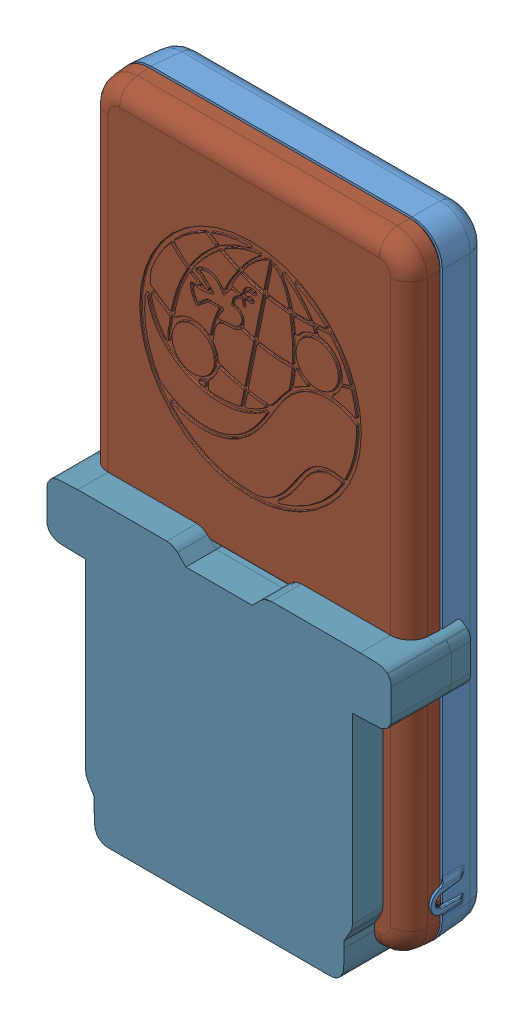
SolidWorks assembly pcb assm new, configuration Default. Lengths in mm.
Overall size (86.92 165.02 40.71).
43 component instances, 14 part files, 21 mates.
Components (placement in the parent):
- pcb top new-1: pcb top new [Default] at origin size (86.92 165 16.48)
- pcb w pot-1: pcb w pot [Default] at (-73.5 149.8449 0.1) x (0 -1 0) z (0 0 -1) size (61 49 35.64)
  - pcb w pot.step-1: pcb w pot.step [Default] at origin size (61 49 48.39)
    - DIP-8_W7.62mm.step-1: DIP-8_W7.62mm.step [Default] at (118.872 -61.849 1.65) x (0 -1 0) z (0 0 1) size (7.87 9.27 6.98)
      - SOLID.step-1: SOLID.step [Default] at origin size (7.87 9.27 6.98)
    - PTV09A-4030S-A503.step-1: PTV09A-4030S-A503.step [Default] at (115.189 -83.439 1.65) x (0 1 0) z (0 0 1) size (11.44 12.9 35.6)
      - COMPOUND.step-1: COMPOUND.step [Default] at origin size (11.44 12.9 35.6)
    - R_0805_2012Metric.step-1: R_0805_2012Metric.step [Default] at (112.411 -57.658 1.65) size (2 1.2 0.45)
      - SOLID-0.step-1: SOLID-0.step [Default] at origin size (2 1.2 0.45)
    - R_0805_2012Metric.step-2: R_0805_2012Metric.step [Default] at (121.682 -90.932 1.65) x (0 -1 0) z (0 0 1) size (2 1.2 0.45)
      - SOLID-0.step-1: SOLID-0.step [Default] at origin size (2 1.2 0.45)
    - R_0805_2012Metric.step-3: R_0805_2012Metric.step [Default] at (121.142 -85.979 1.65) x (-1 0 0) z (0 0 1) size (2 1.2 0.45)
      - SOLID-0.step-1: SOLID-0.step [Default] at origin size (2 1.2 0.45)
    - R_0805_2012Metric.step-4: R_0805_2012Metric.step [Default] at (117.364 -57.658 1.65) size (2 1.2 0.45)
      - SOLID-0.step-1: SOLID-0.step [Default] at origin size (2 1.2 0.45)
    - R_0805_2012Metric.step-5: R_0805_2012Metric.step [Default] at (127 -80.772 1.65) x (-1 0 0) z (0 0 1) size (2 1.2 0.45)
      - SOLID-0.step-1: SOLID-0.step [Default] at origin size (2 1.2 0.45)
    - R_Axial_DIN0207_L6.3mm_D2.5mm_P7.62mm_Horizontal.step-1: R_Axial_DIN0207_L6.3mm_D2.5mm_P7.62mm_Horizontal.step [Default] at (105.537 -92.583 1.65) size (8.22 2.5 5.5)
      - SOLID-1.step-1: SOLID-1.step [Default] at origin size (8.22 2.5 5.5)
    - R_0805_2012Metric.step-6: R_0805_2012Metric.step [Default] at (88.265 -82.534 1.65) x (0 -1 0) z (0 0 1) size (2 1.2 0.45)
      - SOLID-0.step-1: SOLID-0.step [Default] at origin size (2 1.2 0.45)
    - R_Axial_DIN0204_L3.6mm_D1.6mm_P2.54mm_Vertical.step-1: R_Axial_DIN0204_L3.6mm_D1.6mm_P2.54mm_Vertical.step [Default] at (137.668 -93.726 1.65) x (0 1 0) z (0 0 1) size (3.59 1.6 9.6)
      - SOLID-2.step-1: SOLID-2.step [Default] at origin size (3.59 1.6 9.6)
    - R_Axial_DIN0204_L3.6mm_D1.6mm_P2.54mm_Vertical.step-2: R_Axial_DIN0204_L3.6mm_D1.6mm_P2.54mm_Vertical.step [Default] at (132.334 -91.44 1.65) x (0 -1 0) z (0 0 1) size (3.59 1.6 9.6)
      - SOLID-2.step-1: SOLID-2.step [Default] at origin size (3.59 1.6 9.6)
    - LM317MABTG.step-1: LM317MABTG.step [Default] at (95.377 -83.058 1.65) x (0 1 0) z (0 0 1) size (9.97 4.82 36.27)
      - COMPOUND-3.step-1: COMPOUND-3.step [Default] at origin size (9.97 4.82 36.27)
    - C_0805_2012Metric.step-1: C_0805_2012Metric.step [Default] at (118.364 -95.25 1.65) x (0 -1 0) z (0 0 1) size (2 1.25 1.25)
      - SOLID-4.step-1: SOLID-4.step [Default] at origin size (2 1.25 1.25)
    - C_0805_2012Metric.step-2: C_0805_2012Metric.step [Default] at (109.855 -52.832 1.65) x (0 1 0) z (0 0 1) size (2 1.25 1.25)
      - SOLID-4.step-1: SOLID-4.step [Default] at origin size (2 1.25 1.25)
    - C_1206_3216Metric.step-1: C_1206_3216Metric.step [Default] at (121.285 -80.772 1.65) x (-1 0 0) z (0 0 1) size (3.2 1.6 1.6)
      - SOLID-5.step-1: SOLID-5.step [Default] at origin size (3.2 1.6 1.6)
    - C_0805_2012Metric.step-3: C_0805_2012Metric.step [Default] at (88.392 -76.3485 1.65) x (0 1 0) z (0 0 1) size (2 1.25 1.25)
      - SOLID-4.step-1: SOLID-4.step [Default] at origin size (2 1.25 1.25)
    - COMPOUND-6.step-1: COMPOUND-6.step [Default] at origin size (61 49 1.6)
- pcb bottom new-1: pcb bottom new [Default] at origin size (86.85 165 8.73)
- battery case-1: battery case [Default] at (0 -42.734 -10) size (59.56 61.47 15.11)
- Batteria ricaricabile stilo-1: Batteria ricaricabile stilo [Default] at (23.86 -20.0965 -1.9855) x (0 0 1) z (-1 0 0) size (13.97 13.97 50.04)
- Batteria ricaricabile stilo-2: Batteria ricaricabile stilo [Default] at (-23.86 -35.162 -1.9855) x (0 0 -1) z (1 0 0) size (13.97 13.97 50.04)
- Batteria ricaricabile stilo-3: Batteria ricaricabile stilo [Default] at (23.86 -50.2275 -1.872) x (0 0 1) z (-1 0 0) size (13.97 13.97 50.04)
- Batteria ricaricabile stilo-4: Batteria ricaricabile stilo [Default] at (-23.86 -65.3715 -1.9855) x (0 0 -1) z (1 0 0) size (13.97 13.97 50.04)
- pcb battery cover-1: pcb battery cover [Default] at origin size (91.07 78.3 21.02)
Mates (geometry in assembly coordinates):
- Coincident1: coincident anti-aligned: plane of pcb top new-1 through (0 0 -1.6) normal (0 0 1); plane of pcb w pot-1/pcb w pot.step-1/COMPOUND-6.step-1 through (0 36.3711 0) normal (0 0 1)
- Coincident2: coincident anti-aligned: plane of pcb top new-1 through (0 0 -1.5) normal (0 0 1); plane of pcb w pot-1/pcb w pot.step-1/COMPOUND-6.step-1 through (0 36.3449 -1.5) normal (0 0 -1)
- Width4: width aligned: plane of pcb bottom new-1 through (42.5 -82.5 0) normal (0.99863 0 0.052336); plane of pcb top new-1 through (-42.5 -82.5 0) normal (-0.99863 0 0.052336); plane of pcb bottom new-1 through (42.5 -82.5 0) normal (0.99863 0 -0.052336); plane of pcb top new-1 through (-42.5 -82.5 0) normal (-0.99863 0 -0.052336)
- Width5: width anti-aligned: plane of pcb bottom new-1 through (42.5 82.5 0) normal (0 0.99863 0.052336); plane of pcb top new-1 through (42.5 -82.5 0) normal (0 -0.99863 0.052336); plane of pcb bottom new-1 through (42.5 -82.5 0) normal (0 -0.99863 -0.052336); plane of pcb top new-1 through (42.5 82.5 0) normal (0 0.99863 -0.052336)
- Coincident3: coincident anti-aligned: plane of pcb top new-1 through (0 0 0) normal (0 0 1); plane of pcb bottom new-1 through (0 0 0) normal (0 0 -1)
- Width6: width aligned: plane of pcb w pot-1/pcb w pot.step-1/COMPOUND-6.step-1 through (-24.5 5.8449 0.1) normal (0 -1 0); plane of pcb top new-1 through (24.5 66.8449 0.1) normal (0 1 0); plane of pcb w pot-1/pcb w pot.step-1/COMPOUND-6.step-1 through (25.25 5.0949 -1.5) normal (0 0.99863 0.052336); plane of pcb top new-1 through (25.25 67.5949 -1.5) normal (0 -0.99863 0.052336)
- Width7: width aligned: plane of pcb w pot-1/pcb w pot.step-1/COMPOUND-6.step-1 through (24.5 5.8449 0.1) normal (1 0 0); plane of pcb top new-1 through (-24.5 66.8449 0.1) normal (-1 0 0); plane of pcb w pot-1/pcb w pot.step-1/COMPOUND-6.step-1 through (25.25 61.7904 -1.5) normal (-0.99863 0 0.052336); plane of pcb top new-1 through (-25.25 5.0949 -1.5) normal (0.99863 0 0.052336)
- Width8: width aligned: plane of battery case-1 through (-28.448 -12 5.113) normal (-1 0 0); plane of pcb top new-1 through (28.448 -12 5.113) normal (1 0 0); plane of battery case-1 through (42.5 -82.5 0) normal (0.99863 0 -0.052336); plane of pcb top new-1 through (-42.5 -82.5 0) normal (-0.99863 0 -0.052336)
- Coincident4: coincident anti-aligned: plane of pcb top new-1 through (0 0 -10) normal (0 0 1); plane of battery case-1 through (-28.448 -73.468 -10) normal (0 0 -1)
- Concentric1: concentric anti-aligned: cylinder of battery case-1 through (-25.543 -20.0965 -1.9855) axis (-1 0 0) radius 2.77; cylinder of Batteria ricaricabile stilo-1 through (-23.511 -20.0965 -1.9855) axis (1 0 0) radius 6.985
- Coincident5: coincident anti-aligned: circle of battery case-1; plane of Batteria ricaricabile stilo-1 through (-25.543 -20.0965 -1.9855) normal (-1 0 0)
- Concentric2: concentric anti-aligned: cylinder of battery case-1 through (25.543 -35.162 -1.9855) axis (1 0 0) radius 2.75; cylinder of Batteria ricaricabile stilo-2 through (23.511 -35.162 -1.9855) axis (-1 0 0) radius 6.985
- Coincident6: coincident anti-aligned: circle of battery case-1; plane of Batteria ricaricabile stilo-2 through (25.543 -35.162 -1.9855) normal (1 0 0)
- Concentric3: concentric anti-aligned: cylinder of battery case-1 through (-25.543 -50.2275 -1.872) axis (-1 0 0) radius 2.75; cylinder of Batteria ricaricabile stilo-3 through (-23.511 -50.2275 -1.872) axis (1 0 0) radius 6.985
- Coincident7: coincident anti-aligned: circle of battery case-1; plane of Batteria ricaricabile stilo-3 through (-25.543 -50.2275 -1.872) normal (-1 0 0)
- Concentric4: concentric anti-aligned: cylinder of battery case-1 through (-49.403 -65.3715 -1.9855) axis (1 0 0) radius 1.27; cylinder of Batteria ricaricabile stilo-4 through (23.511 -65.3715 -1.9855) axis (-1 0 0) radius 6.985
- Coincident8: coincident aligned: plane of Batteria ricaricabile stilo-2 through (25.543 -35.162 -1.9855) normal (1 0 0); plane of Batteria ricaricabile stilo-4 through (25.543 -65.3715 -1.9855) normal (1 0 0)
- Distance1: distance = 12 mm aligned: line of battery case-1; plane of assembly through (0 0 0) normal (0 1 0)
- Width10: width anti-aligned: plane of pcb battery cover-1 through (-42.4694 -19 0.5847) normal (-0.99863 0 0.052336); plane of pcb battery cover-1 through (42.3029 -19 3.7617) normal (0.99863 0 0.052336); plane of pcb top new-1 through (42.5 -82.5 0) normal (0.99863 0 -0.052336); plane of pcb top new-1 through (-42.5 -82.5 0) normal (-0.99863 0 -0.052336)
- Coincident10: coincident anti-aligned: plane of pcb bottom new-1 through (37.3097 -20 7.25) normal (0 0 1); plane of pcb battery cover-1 through (33.1646 -19 7.25) normal (0 0 -1)
- Width11: width aligned: plane of pcb battery cover-1 through (-42.4694 -19 0.5847) normal (0 -0.99863 -0.052336); plane of pcb battery cover-1 through (-42.4694 -11 0.5847) normal (0 0.99863 -0.052336); plane of pcb bottom new-1 through (42.5104 -12.535 0.014) normal (0 -0.984767 -0.173879); plane of pcb bottom new-1 through (42.7789 -16.5604 5.1373) normal (0 0.984767 -0.173879)
